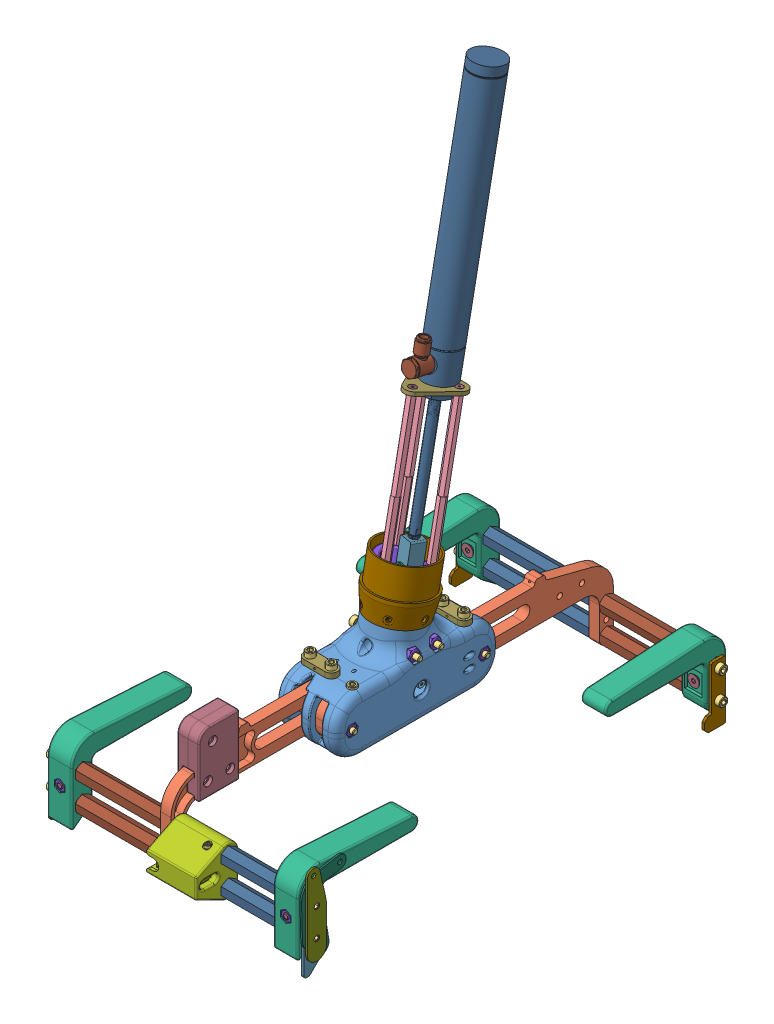
SolidWorks assembly 971-18-A-4000_The Claw, configuration Default. Lengths in mm. (continued)
Mates (geometry in assembly coordinates): (continued)
- Concentric85: concentric anti-aligned: cylinder of 971-18-P-0153_Claw Piston Mount-1 through (0 214.9449 -23.313) axis (0 0.981514 -0.19139) radius 1.632; cylinder of FHCS-19 through (0 208.7122 -22.0976) axis (0 -0.981514 0.19139) radius 1.4224
- Coincident109: coincident aligned: plane of 971-18-P-0153_Claw Piston Mount-1 through (-15.7499 209.7238 -50.0883) normal (0 0.981514 -0.19139); plane of FHCS-19 through (-1.3527 214.8607 -23.7448) normal (0 0.981514 -0.19139)
- Concentric90: concentric anti-aligned: cylinder of Bearings-1 through (15.2468 27.94 -18.3873) axis (1 0 0) radius 4.7625; cylinder of 971-18-P-0120_Printed Claw Pulley-4 through (0.264 27.94 -18.3873) axis (-1 0 0) radius 4.7625
- Coincident116: coincident anti-aligned: plane of Bearings-1 through (7.7788 27.5507 -23.1339) normal (-1 0 0); plane of 971-18-P-0120_Printed Claw Pulley-4 through (7.7788 31.7428 -18.1529) normal (1 0 0)
- Coincident117: coincident anti-aligned: plane of Bearings-2 through (-11.0808 23.5364 -0.7924) normal (-1 0 0); plane of 971-18-P-0120_Printed Claw Pulley-3 through (-11.0808 29.7802 -2.3147) normal (1 0 0)
- Concentric91: concentric anti-aligned: cylinder of Bearings-2 through (-3.6127 27.94 1.0215) axis (1 0 0) radius 4.7625; cylinder of 971-18-P-0120_Printed Claw Pulley-3 through (-18.5955 27.94 1.0215) axis (-1 0 0) radius 4.7625
- Concentric1168: concentric aligned: cone of 971-18-P-0108_Printed Claw Body-1 through (-11.1125 53.5447 9.169) axis (0.5 -0.165748 -0.850016); cone of 93365A142_BRASS HEAT-SET INSERT FOR PLASTICS-1 through (-10.8148 53.446 8.663) axis (0.5 -0.165748 -0.850016)
- Tangent1: tangent aligned: cylinder of 971-18-P-0108_Printed Claw Body-1 through (0 43.6283 -8.5073) axis (0 0.981514 -0.19139) radius 22.225; plane of 93365A142_BRASS HEAT-SET INSERT FOR PLASTICS-1 through (-11.1125 53.5447 9.169) normal (-0.5 0.165748 0.850016)
- Concentric1169: concentric aligned: cone of 971-18-P-0108_Printed Claw Body-1 through (-22.225 49.8609 -9.7226) axis (1 0 0); cone of 93365A142_BRASS HEAT-SET INSERT FOR PLASTICS-2 through (-21.6297 49.8609 -9.7226) axis (1 0 0)
- Tangent2: tangent aligned: cylinder of 971-18-P-0108_Printed Claw Body-1 through (0 43.6283 -8.5073) axis (0 0.981514 -0.19139) radius 22.225; plane of 93365A142_BRASS HEAT-SET INSERT FOR PLASTICS-2 through (-22.225 49.8609 -9.7226) normal (-1 0 0)
- Concentric1170: concentric aligned: cone of 971-18-P-0108_Printed Claw Body-1 through (-11.1125 46.1772 -28.6142) axis (0.5 0.165748 0.850016); cone of 93365A142_BRASS HEAT-SET INSERT FOR PLASTICS-4 through (-10.8148 46.2758 -28.1082) axis (0.5 0.165748 0.850016)
- Tangent3: tangent aligned: cylinder of 971-18-P-0108_Printed Claw Body-1 through (0 43.6283 -8.5073) axis (0 0.981514 -0.19139) radius 22.225; plane of 93365A142_BRASS HEAT-SET INSERT FOR PLASTICS-4 through (-11.1125 46.1772 -28.6142) normal (-0.5 -0.165748 -0.850016)
- Concentric1171: concentric aligned: cone of 971-18-P-0108_Printed Claw Body-1 through (11.1125 46.1772 -28.6142) axis (-0.5 0.165748 0.850016); cone of 93365A142_BRASS HEAT-SET INSERT FOR PLASTICS-6 through (10.8148 46.2758 -28.1082) axis (-0.5 0.165748 0.850016)
- Tangent4: tangent aligned: cylinder of 971-18-P-0108_Printed Claw Body-1 through (0 43.6283 -8.5073) axis (0 0.981514 -0.19139) radius 22.225; plane of 93365A142_BRASS HEAT-SET INSERT FOR PLASTICS-6 through (11.1125 46.1772 -28.6142) normal (0.5 -0.165748 -0.850016)
- Concentric1172: concentric aligned: cone of 971-18-P-0108_Printed Claw Body-1 through (22.225 49.8609 -9.7226) axis (-1 0 0); cone of 93365A142_BRASS HEAT-SET INSERT FOR PLASTICS-8 through (21.6297 49.8609 -9.7226) axis (-1 0 0)
- Tangent5: tangent aligned: cylinder of 971-18-P-0108_Printed Claw Body-1 through (0 43.6283 -8.5073) axis (0 0.981514 -0.19139) radius 22.225; plane of 93365A142_BRASS HEAT-SET INSERT FOR PLASTICS-8 through (22.225 49.8609 -9.7226) normal (1 0 0)
- Concentric1173: concentric aligned: cone of 971-18-P-0108_Printed Claw Body-1 through (11.1125 53.5447 9.169) axis (-0.5 -0.165748 -0.850016); cone of 93365A142_BRASS HEAT-SET INSERT FOR PLASTICS-10 through (10.8148 53.446 8.663) axis (-0.5 -0.165748 -0.850016)
- Tangent6: tangent aligned: cylinder of 971-18-P-0108_Printed Claw Body-1 through (0 43.6283 -8.5073) axis (0 0.981514 -0.19139) radius 22.225; plane of 93365A142_BRASS HEAT-SET INSERT FOR PLASTICS-10 through (11.1125 53.5447 9.169) normal (0.5 0.165748 0.850016)
- Tangent7: tangent: cylinder of 971-18-P-0108_Printed Claw Body-1 through (-25.2095 0 36.5125) axis (1 0 0) radius 3.175; torus of 9433K640_PRECISION STAINLESS STEEL EXTENSION SPRING-2
- Concentric1202: concentric anti-aligned: circle of 92311A433_18-8 SS CUP POINT SET SCREW-11; circle of 971-18-P-0077_Main Claw plate-2
- Concentric1206: concentric anti-aligned: circle of 92311A433_18-8 SS CUP POINT SET SCREW-14; circle of 971-18-P-0077_Main Claw plate-2
- Concentric1207: concentric anti-aligned: circle of SHCS-43; circle of 92311A433_18-8 SS CUP POINT SET SCREW-11
- Concentric1215: concentric anti-aligned: cylinder of SHCS-12 through (-19.177 30.1625 50.8) axis (0 -1 0) radius 2.413; circle of 94638A222_NYLON UNTHREADED SPACERS-1
- Width22: width anti-aligned: plane of 94638A222_NYLON UNTHREADED SPACERS-1 through (-19.177 16.6687 50.8) normal (0 1 0); plane of 971-18-P-0108_Printed Claw Body-1 through (-19.177 -16.6687 50.8) normal (0 -1 0); plane of 94638A222_NYLON UNTHREADED SPACERS-1 through (3.81 17.4625 -74.6125) normal (0 -1 0); plane of 971-18-P-0108_Printed Claw Body-1 through (3.81 -17.4625 -74.6125) normal (0 1 0)
- Concentric1216: concentric anti-aligned: cylinder of SHCS-3 through (-19.177 22.225 -50.8) axis (0 -1 0) radius 2.413; circle of 94638A222_NYLON UNTHREADED SPACERS-2
- Width23: width anti-aligned: plane of 94638A222_NYLON UNTHREADED SPACERS-2 through (-19.177 16.6687 -50.8) normal (0 1 0); plane of 971-18-P-0108_Printed Claw Body-1 through (-19.177 -16.6687 -50.8) normal (0 -1 0); plane of 94638A222_NYLON UNTHREADED SPACERS-2 through (3.81 17.4625 -74.6125) normal (0 -1 0); plane of 971-18-P-0108_Printed Claw Body-1 through (3.81 -17.4625 -74.6125) normal (0 1 0)
- Concentric1217: concentric anti-aligned: cylinder of SHCS-11 through (0 30.1625 50.8) axis (0 -1 0) radius 2.413; circle of 94639A586_NYLON UNTHREADED SPACERS-3
- Width25: width anti-aligned: plane of 94639A586_NYLON UNTHREADED SPACERS-3 through (0 -6.7469 50.8) normal (0 1 0); plane of 971-18-P-0108_Printed Claw Body-1 through (0 -17.0656 50.8) normal (0 -1 0); plane of 94639A586_NYLON UNTHREADED SPACERS-3 through (0 -6.35 50.8) normal (0 -1 0); plane of 971-18-P-0108_Printed Claw Body-1 through (3.81 -17.4625 -74.6125) normal (0 1 0)
- Concentric1218: concentric anti-aligned: cylinder of SHCS-11 through (0 30.1625 50.8) axis (0 -1 0) radius 2.413; circle of 94639A586_NYLON UNTHREADED SPACERS-1
- Width26: width anti-aligned: plane of 94639A586_NYLON UNTHREADED SPACERS-1 through (0 17.0656 50.8) normal (0 1 0); plane of 971-18-P-0108_Printed Claw Body-1 through (0 6.7469 50.8) normal (0 -1 0); plane of 94639A586_NYLON UNTHREADED SPACERS-1 through (3.81 17.4625 -74.6125) normal (0 -1 0); plane of 971-18-P-0108_Printed Claw Body-1 through (0 6.35 50.8) normal (0 1 0)
- Concentric1219: concentric anti-aligned: cylinder of SHCS-8 through (0 30.1625 -50.8) axis (0 -1 0) radius 2.413; circle of 94639A586_NYLON UNTHREADED SPACERS-4
- Width27: width aligned: plane of 94639A586_NYLON UNTHREADED SPACERS-4 through (0 -6.7469 -50.8) normal (0 1 0); plane of 971-18-P-0108_Printed Claw Body-1 through (0 -17.0656 -50.8) normal (0 -1 0); plane of 94639A586_NYLON UNTHREADED SPACERS-4 through (3.81 -17.4625 -74.6125) normal (0 1 0); plane of 971-18-P-0108_Printed Claw Body-1 through (0 -6.35 -50.8) normal (0 -1 0)
- Concentric1220: concentric anti-aligned: cylinder of SHCS-8 through (0 30.1625 -50.8) axis (0 -1 0) radius 2.413; circle of 94639A586_NYLON UNTHREADED SPACERS-2
- Width28: width anti-aligned: plane of 94639A586_NYLON UNTHREADED SPACERS-2 through (0 17.0656 -50.8) normal (0 1 0); plane of 971-18-P-0108_Printed Claw Body-1 through (0 6.7469 -50.8) normal (0 -1 0); plane of 94639A586_NYLON UNTHREADED SPACERS-2 through (3.81 17.4625 -74.6125) normal (0 -1 0); plane of 971-18-P-0108_Printed Claw Body-1 through (0 6.35 -50.8) normal (0 1 0)
- Concentric1221: concentric anti-aligned: cylinder of SHCS-10 through (19.177 22.225 50.8) axis (0 -1 0) radius 2.413; circle of 94638A222_NYLON UNTHREADED SPACERS-4
- Concentric1222: concentric anti-aligned: cylinder of SHCS-9 through (19.177 30.1625 -50.8) axis (0 -1 0) radius 2.413; circle of 94638A222_NYLON UNTHREADED SPACERS-3
- Width29: width anti-aligned: plane of 94638A222_NYLON UNTHREADED SPACERS-3 through (19.177 16.6687 -50.8) normal (0 1 0); plane of 971-18-P-0108_Printed Claw Body-1 through (19.177 -16.6687 -50.8) normal (0 -1 0); plane of 94638A222_NYLON UNTHREADED SPACERS-3 through (3.81 17.4625 -74.6125) normal (0 -1 0); plane of 971-18-P-0108_Printed Claw Body-1 through (3.81 -17.4625 -74.6125) normal (0 1 0)
- Width30: width anti-aligned: plane of 94638A222_NYLON UNTHREADED SPACERS-4 through (19.177 -16.6687 50.8) normal (0 -1 0); plane of 971-18-P-0108_Printed Claw Body-1 through (19.177 16.6687 50.8) normal (0 1 0); plane of 94638A222_NYLON UNTHREADED SPACERS-4 through (3.81 -17.4625 -74.6125) normal (0 1 0); plane of 971-18-P-0108_Printed Claw Body-1 through (3.81 17.4625 -74.6125) normal (0 -1 0)
- Concentric1223: concentric anti-aligned: cylinder of SHCS-2 through (-25.4 0 60.325) axis (1 0 0) radius 2.413; circle of 94639A550_NYLON UNTHREADED SPACERS-3
- Width31: width anti-aligned: plane of 94639A550_NYLON UNTHREADED SPACERS-3 through (-4.6673 0 60.325) normal (1 0 0); plane of 971-18-P-0108_Printed Claw Body-1 through (-14.1922 0 60.325) normal (-1 0 0); plane of 94639A550_NYLON UNTHREADED SPACERS-3 through (-3.81 17.4625 -74.6125) normal (-1 0 0); plane of 971-18-P-0108_Printed Claw Body-1 through (-15.0495 17.4625 -74.6125) normal (1 0 0)
- Concentric1224: concentric anti-aligned: cylinder of SHCS-2 through (-25.4 0 60.325) axis (1 0 0) radius 2.413; circle of 94639A550_NYLON UNTHREADED SPACERS-4
- Width32: width anti-aligned: plane of 94639A550_NYLON UNTHREADED SPACERS-4 through (4.6673 0 60.325) normal (-1 0 0); plane of 971-18-P-0108_Printed Claw Body-1 through (14.1922 0 60.325) normal (1 0 0); plane of 94639A550_NYLON UNTHREADED SPACERS-4 through (3.81 17.4625 -74.6125) normal (1 0 0); plane of 971-18-P-0108_Printed Claw Body-1 through (15.0495 17.4625 -74.6125) normal (-1 0 0)
- Concentric1225: concentric aligned: cylinder of SHCS-1 through (-25.4 0 -60.325) axis (1 0 0) radius 2.413; circle of 94639A550_NYLON UNTHREADED SPACERS-1
- Width33: width anti-aligned: plane of 94639A550_NYLON UNTHREADED SPACERS-1 through (-14.1922 0 -60.325) normal (-1 0 0); plane of 971-18-P-0108_Printed Claw Body-1 through (-4.6673 0 -60.325) normal (1 0 0); plane of 94639A550_NYLON UNTHREADED SPACERS-1 through (-15.0495 17.4625 -74.6125) normal (1 0 0); plane of 971-18-P-0108_Printed Claw Body-1 through (-3.81 17.4625 -74.6125) normal (-1 0 0)
- Concentric1226: concentric anti-aligned: cylinder of SHCS-1 through (-25.4 0 -60.325) axis (1 0 0) radius 2.413; circle of 94639A550_NYLON UNTHREADED SPACERS-2
- Width34: width aligned: plane of 94639A550_NYLON UNTHREADED SPACERS-2 through (4.6673 0 -60.325) normal (-1 0 0); plane of 971-18-P-0108_Printed Claw Body-1 through (14.1922 0 -60.325) normal (1 0 0); plane of 94639A550_NYLON UNTHREADED SPACERS-2 through (15.0495 17.4625 -74.6125) normal (-1 0 0); plane of 971-18-P-0108_Printed Claw Body-1 through (3.81 17.4625 -74.6125) normal (1 0 0)
- Concentric1236: concentric aligned: circle of 971-18-P-0077_Main Claw plate-3; circle of 92311A433_18-8 SS CUP POINT SET SCREW-5
- Concentric1238: concentric anti-aligned: circle of 971-18-P-0077_Main Claw plate-3; circle of 92311A433_18-8 SS CUP POINT SET SCREW-1
- Concentric1275: concentric aligned: circle of 91780A049_ALUM FEM THRDED HEX STANDOFF-2; circle of 98637A123_ALLOY STEEL MIL SPEC CUP POINT SET SCREW-3
- Concentric1276: concentric aligned: circle of 91780A049_ALUM FEM THRDED HEX STANDOFF-5; circle of 98637A123_ALLOY STEEL MIL SPEC CUP POINT SET SCREW-3
- Coincident286: coincident anti-aligned: plane of 91780A049_ALUM FEM THRDED HEX STANDOFF-2 through (17.26 132.4555 -31.6177) normal (0 0.981514 -0.19139); plane of 91780A049_ALUM FEM THRDED HEX STANDOFF-5 through (18.7431 132.2213 -32.8189) normal (0 -0.981514 0.19139)
- Concentric1277: concentric anti-aligned: circle of 91780A049_ALUM FEM THRDED HEX STANDOFF-3; circle of 98637A123_ALLOY STEEL MIL SPEC CUP POINT SET SCREW-2
- Concentric1278: concentric aligned: circle of 91780A049_ALUM FEM THRDED HEX STANDOFF-4; circle of 98637A123_ALLOY STEEL MIL SPEC CUP POINT SET SCREW-2
- Coincident287: coincident anti-aligned: plane of 91780A049_ALUM FEM THRDED HEX STANDOFF-3 through (-15.7499 131.1145 -38.4951) normal (0 -0.981514 0.19139); plane of 91780A049_ALUM FEM THRDED HEX STANDOFF-4 through (-12.0838 131.8123 -34.9162) normal (0 0.981514 -0.19139)
- Concentric1279: concentric anti-aligned: circle of 98637A123_ALLOY STEEL MIL SPEC CUP POINT SET SCREW-1; circle of 91780A049_ALUM FEM THRDED HEX STANDOFF-6
- Concentric1280: concentric anti-aligned: circle of 91780A049_ALUM FEM THRDED HEX STANDOFF-1; circle of 98637A123_ALLOY STEEL MIL SPEC CUP POINT SET SCREW-1
- Coincident289: coincident anti-aligned: plane of 91780A049_ALUM FEM THRDED HEX STANDOFF-1 through (-3.5893 137.1801 -7.3885) normal (0 -0.981514 0.19139); plane of 91780A049_ALUM FEM THRDED HEX STANDOFF-6 through (1.8331 137.6448 -5.0051) normal (0 0.981514 -0.19139)
- Concentric1281: concentric anti-aligned: cylinder of FHCS-17 through (0 208.7122 -22.0976) axis (0 -0.981514 0.19139) radius 1.4224; circle of 91780A049_ALUM FEM THRDED HEX STANDOFF-6
- Coincident291: coincident anti-aligned: plane of 971-18-P-0153_Claw Piston Mount-1 through (-15.7499 206.6075 -49.4806) normal (0 -0.981514 0.19139); plane of 91780A049_ALUM FEM THRDED HEX STANDOFF-1 through (-3.5893 211.9715 -21.9724) normal (0 0.981514 -0.19139)
- Concentric1282: concentric anti-aligned: circle of FHCS-18; circle of 91780A049_ALUM FEM THRDED HEX STANDOFF-5
- Coincident293: coincident anti-aligned: plane of 971-18-P-0153_Claw Piston Mount-1 through (-15.7499 206.6075 -49.4806) normal (0 -0.981514 0.19139); plane of 91780A049_ALUM FEM THRDED HEX STANDOFF-5 through (18.7431 207.0127 -47.4028) normal (0 0.981514 -0.19139)
- Concentric1283: concentric anti-aligned: circle of FHCS-15; circle of 91780A049_ALUM FEM THRDED HEX STANDOFF-3
- Coincident294: coincident anti-aligned: plane of 971-18-P-0153_Claw Piston Mount-1 through (-15.7499 206.6075 -49.4806) normal (0 -0.981514 0.19139); plane of 91780A049_ALUM FEM THRDED HEX STANDOFF-3 through (-15.7499 205.9058 -53.079) normal (0 0.981514 -0.19139)
- Concentric1310: concentric anti-aligned: cylinder of Beam Diffuse Sensor-1 through (30.5617 -48.646 194.183) axis (0 1 0) radius 1.524; cylinder of SHCS-26 through (30.5617 -24.389 194.183) axis (0 -1 0) radius 1.4224
- Concentric1313: concentric aligned: cylinder of 94639A550_NYLON UNTHREADED SPACERS-4 through (4.6673 0 60.325) axis (1 0 0) radius 6.35; cylinder of 94639A550_NYLON UNTHREADED SPACERS-3 through (-14.1922 0 60.325) axis (1 0 0) radius 6.35
- Concentric1314: concentric aligned: cylinder of SHCS-37 through (116.3637 -29.5056 -185.7375) axis (-1 0 0) radius 2.413; cylinder of 971-18-P-0299_Printed Claw Ends-1 through (114.0778 -29.5056 -185.7375) axis (-1 0 0) radius 2.4892
- Concentric1315: concentric aligned: cylinder of SHCS-39 through (116.3637 -54.9056 -185.7375) axis (-1 0 0) radius 2.413; cylinder of 971-18-P-0299_Printed Claw Ends-1 through (114.0778 -54.9056 -185.7375) axis (-1 0 0) radius 2.4892
- Concentric1316: concentric anti-aligned: cylinder of SHCS-43 through (-116.3637 -29.5056 -185.7375) axis (1 0 0) radius 2.413; cylinder of 971-18-P-0299_Printed Claw Ends-2 through (-91.8528 -29.5056 -185.7375) axis (-1 0 0) radius 2.4892
- Concentric1317: concentric anti-aligned: cylinder of SHCS-41 through (-116.3637 -54.9056 -185.7375) axis (1 0 0) radius 2.413; cylinder of 971-18-P-0299_Printed Claw Ends-2 through (-91.8528 -54.9056 -185.7375) axis (-1 0 0) radius 2.4892
- Concentric1318: concentric aligned: cylinder of SHCS-24 through (-116.3637 -29.5056 185.7375) axis (1 0 0) radius 2.413; cylinder of 971-18-P-0299_Printed Claw Ends-3 through (-114.0778 -29.5056 185.7375) axis (1 0 0) radius 2.4892
- Concentric1319: concentric aligned: cylinder of SHCS-44 through (-116.3637 -54.9056 185.7375) axis (1 0 0) radius 2.413; cylinder of 971-18-P-0299_Printed Claw Ends-3 through (-114.0778 -54.9056 185.7375) axis (1 0 0) radius 2.4892
- Concentric1321: concentric anti-aligned: cylinder of SHCS-33 through (116.3637 -29.5056 185.7375) axis (-1 0 0) radius 2.413; cylinder of 971-18-P-0299_Printed Claw Ends-4 through (91.8528 -29.5056 185.7375) axis (1 0 0) radius 2.4892
- Concentric1322: concentric anti-aligned: cylinder of SHCS-35 through (116.3637 -54.9056 185.7375) axis (-1 0 0) radius 2.413; cylinder of 971-18-P-0299_Printed Claw Ends-4 through (91.8528 -54.9056 185.7375) axis (1 0 0) radius 2.4892
- Coincident363: coincident anti-aligned: plane of 971-18-P-0077_Main Claw plate-3 through (-4.6673 -158.75 26.9875) normal (1 0 0); plane of 971-18-P-0300_Printed Claw Beam Break Mount-1 through (-4.6673 -29.469 185.801) normal (-1 0 0)
- Coincident365: coincident anti-aligned: plane of Beam Diffuse Sensor-1 through (2.3678 -48.646 191.135) normal (0 0 -1); plane of 971-18-P-0300_Printed Claw Beam Break Mount-1 through (-4.6673 -35.692 191.135) normal (0 0 1)
- Coincident366: coincident anti-aligned: plane of Beam Diffuse Sensor-1 through (2.3678 -48.646 191.135) normal (0 -1 0); plane of 971-18-P-0300_Printed Claw Beam Break Mount-1 through (-4.6673 -48.646 191.135) normal (0 1 0)
- Coincident367: coincident anti-aligned: plane of Beam Diffuse Sensor-1 through (34.0678 -48.646 212.217) normal (1 0 0); plane of 971-18-P-0300_Printed Claw Beam Break Mount-1 through (34.0678 -35.819 225.3308) normal (-1 0 0)
- Coincident368: coincident anti-aligned: plane of SHCS-26 through (31.0198 -24.389 192.0498) normal (0 -1 0); plane of 971-18-P-0300_Printed Claw Beam Break Mount-1 through (30.5626 -24.389 194.183) normal (0 1 0)
- Concentric1324: concentric anti-aligned: cylinder of 971-18-P-0299_Printed Claw Ends-4 through (102.9652 -42.2056 195.2625) axis (0 0 -1) radius 2.4892; cylinder of FHCS-20 through (102.9652 -42.2056 195.2625) axis (0 0 1) radius 2.413
- Concentric1325: concentric anti-aligned: cylinder of Nylon-Insert Locknut-22 through (102.9652 -42.2056 188.087) axis (0 0 -1) radius 2.413; cylinder of FHCS-20 through (102.9652 -42.2056 195.2625) axis (0 0 1) radius 2.413
- Coincident373: coincident anti-aligned: plane of 971-18-P-0299_Printed Claw Ends-4 through (102.9652 -29.5056 190.5) normal (0 0 1); plane of Nylon-Insert Locknut-22 through (103.2706 -47.6964 190.5) normal (0 0 -1)
- Coincident374: coincident aligned: plane of 971-18-P-0299_Printed Claw Ends-4 through (91.8528 -26.9529 176.2125) normal (0 0 -1); plane of FHCS-20 through (103.8895 -44.4346 176.2125) normal (0 0 -1)
- Concentric1327: concentric anti-aligned: cylinder of 971-18-P-0299_Printed Claw Ends-3 through (-102.9652 -42.2056 195.2625) axis (0 0 -1) radius 2.4892; cylinder of FHCS-21 through (-102.9652 -42.2056 195.2625) axis (0 0 1) radius 2.413
- Coincident375: coincident aligned: plane of 971-18-P-0299_Printed Claw Ends-3 through (-114.0778 -26.9529 176.2125) normal (0 0 -1); plane of FHCS-21 through (-101.7917 -44.314 176.2125) normal (0 0 -1)
- Coincident376: coincident aligned: plane of 971-18-P-0299_Printed Claw Ends-2 through (-91.8528 -26.9529 -176.2125) normal (0 0 1); plane of FHCS-24 through (-105.3759 -42.0994 -176.2125) normal (0 0 1)
- Concentric1328: concentric anti-aligned: cylinder of 971-18-P-0299_Printed Claw Ends-2 through (-102.9652 -42.2056 -195.2625) axis (0 0 1) radius 2.4892; cylinder of FHCS-24 through (-102.9652 -42.2056 -195.2625) axis (0 0 -1) radius 2.413
- Concentric1329: concentric anti-aligned: cylinder of 971-18-P-0299_Printed Claw Ends-1 through (102.9652 -42.2056 -195.2625) axis (0 0 1) radius 2.4892; cylinder of FHCS-26 through (102.9652 -42.2056 -195.2625) axis (0 0 -1) radius 2.413
- Coincident377: coincident aligned: plane of 971-18-P-0299_Printed Claw Ends-1 through (114.0778 -26.9529 -176.2125) normal (0 0 1); plane of FHCS-26 through (100.5728 -42.5196 -176.2125) normal (0 0 1)
- Concentric1330: concentric anti-aligned: cylinder of FHCS-21 through (-102.9652 -42.2056 195.2625) axis (0 0 1) radius 2.413; cylinder of Nylon-Insert Locknut-23 through (-102.9652 -42.2056 188.087) axis (0 0 -1) radius 2.413
- Coincident378: coincident anti-aligned: plane of 971-18-P-0299_Printed Claw Ends-3 through (-102.9652 -29.5056 190.5) normal (0 0 1); plane of Nylon-Insert Locknut-23 through (-102.033 -47.6253 190.5) normal (0 0 -1)
- Concentric1331: concentric anti-aligned: cylinder of FHCS-24 through (-102.9652 -42.2056 -195.2625) axis (0 0 -1) radius 2.413; cylinder of Nylon-Insert Locknut-25 through (-102.9652 -42.2056 -188.087) axis (0 0 1) radius 2.413
- Coincident379: coincident anti-aligned: plane of 971-18-P-0299_Printed Claw Ends-2 through (-102.9652 -29.5056 -190.5) normal (0 0 -1); plane of Nylon-Insert Locknut-25 through (-108.2293 -43.7966 -190.5) normal (0 0 1)
- Concentric1332: concentric anti-aligned: cylinder of FHCS-26 through (102.9652 -42.2056 -195.2625) axis (0 0 -1) radius 2.413; cylinder of Nylon-Insert Locknut-27 through (102.9652 -42.2056 -188.087) axis (0 0 1) radius 2.413
- Coincident380: coincident anti-aligned: plane of 971-18-P-0299_Printed Claw Ends-1 through (102.9652 -29.5056 -190.5) normal (0 0 -1); plane of Nylon-Insert Locknut-27 through (98.0574 -44.6866 -190.5) normal (0 0 1)
- Concentric1336: concentric anti-aligned: cylinder of 971-18-P-0108_Printed Claw Body-1 through (0 -22.2934 4.3471) axis (0 0.981514 -0.19139) radius 14.2875; cylinder of 971-18-P-0304_Claw Standoff Ring-1 through (0 84.2529 -16.4288) axis (0 -0.981514 0.19139) radius 15.875
- Coincident388: coincident anti-aligned: plane of 91780A049_ALUM FEM THRDED HEX STANDOFF-6 through (1.8331 62.8535 9.5788) normal (0 0.19139 0.981514); plane of 971-18-P-0304_Claw Standoff Ring-1 through (-1.8331 88.3546 4.6062) normal (0 -0.19139 -0.981514)
- Coincident389: coincident anti-aligned: plane of 91780A049_ALUM FEM THRDED HEX STANDOFF-6 through (-1.8331 62.8535 9.5788) normal (-0.866025 0.095695 0.490757); plane of 971-18-P-0304_Claw Standoff Ring-1 through (-3.6662 87.7469 1.4899) normal (0.866025 -0.095695 -0.490757)
- Concentric1337: concentric anti-aligned: cylinder of 971-18-P-0299_Printed Claw Ends-4 through (91.8528 -29.5056 185.7375) axis (1 0 0) radius 2.4892; cylinder of 971-18-P-0312_Claw Fangs-1 through (116.3637 -29.5056 185.7375) axis (-1 0 0) radius 2.4892
- Concentric1338: concentric anti-aligned: cylinder of 971-18-P-0299_Printed Claw Ends-4 through (91.8528 -54.9056 185.7375) axis (1 0 0) radius 2.4892; cylinder of 971-18-P-0312_Claw Fangs-1 through (116.3637 -54.9056 185.7375) axis (-1 0 0) radius 2.4892
- Coincident390: coincident anti-aligned: plane of 971-18-P-0299_Printed Claw Ends-4 through (114.0778 -54.9056 185.7375) normal (1 0 0); plane of 971-18-P-0312_Claw Fangs-1 through (114.0778 -76.4956 200.7755) normal (-1 0 0)
- Coincident391: coincident anti-aligned: plane of SHCS-33 through (116.3637 -27.5183 188.8835) normal (-1 0 0); plane of 971-18-P-0312_Claw Fangs-1 through (116.3637 -76.4956 200.7755) normal (1 0 0)
- Coincident392: coincident anti-aligned: plane of SHCS-35 through (116.3637 -52.021 183.3869) normal (-1 0 0); plane of 971-18-P-0312_Claw Fangs-1 through (116.3637 -76.4956 200.7755) normal (1 0 0)
- Concentric1342: concentric aligned: cylinder of 971-18-P-0077_Main Claw plate-2 through (14.1922 -54.9056 -185.7375) axis (-1 0 0) radius 2.4892; cylinder of 971-18-P-0299_Printed Claw Ends-1 through (114.0778 -54.9056 -185.7375) axis (-1 0 0) radius 2.4892
- Concentric1344: concentric aligned: cylinder of 971-18-P-0077_Main Claw plate-3 through (-14.1922 -29.5056 185.7375) axis (1 0 0) radius 2.4892; cylinder of SHCS-24 through (-116.3637 -29.5056 185.7375) axis (1 0 0) radius 2.413
- Concentric1347: concentric anti-aligned: cylinder of 971-18-P-0299_Printed Claw Ends-2 through (-91.8528 -29.5056 -185.7375) axis (-1 0 0) radius 2.4892; cylinder of 971-18-P-0312_Claw Fangs-6 through (-116.3637 -29.5056 -185.7375) axis (1 0 0) radius 2.4892
- Concentric1348: concentric anti-aligned: cylinder of 971-18-P-0299_Printed Claw Ends-2 through (-91.8528 -54.9056 -185.7375) axis (-1 0 0) radius 2.4892; cylinder of 971-18-P-0312_Claw Fangs-6 through (-116.3637 -54.9056 -185.7375) axis (1 0 0) radius 2.4892
- Coincident396: coincident anti-aligned: plane of 971-18-P-0299_Printed Claw Ends-2 through (-114.0778 -54.9056 -185.7375) normal (-1 0 0); plane of 971-18-P-0312_Claw Fangs-6 through (-114.0778 -76.4956 -200.7755) normal (1 0 0)
- Coincident397: coincident anti-aligned: plane of SHCS-41 through (-116.3637 -58.3774 -187.0767) normal (1 0 0); plane of 971-18-P-0312_Claw Fangs-6 through (-116.3637 -76.4956 -200.7755) normal (-1 0 0)
- Coincident398: coincident anti-aligned: plane of SHCS-43 through (-116.3637 -28.7687 -189.3849) normal (1 0 0); plane of 971-18-P-0312_Claw Fangs-6 through (-116.3637 -76.4956 -200.7755) normal (-1 0 0)
- Concentric1354: concentric anti-aligned: cylinder of SHCS-37 through (116.3637 -29.5056 -185.7375) axis (-1 0 0) radius 2.413; cylinder of 971-18-P-0312_Claw Fangs-11 through (114.0778 -29.5056 -185.7375) axis (1 0 0) radius 2.4892
- Concentric1355: concentric anti-aligned: cylinder of SHCS-39 through (116.3637 -54.9056 -185.7375) axis (-1 0 0) radius 2.413; cylinder of 971-18-P-0312_Claw Fangs-11 through (114.0778 -54.9056 -185.7375) axis (1 0 0) radius 2.4892
- Coincident406: coincident anti-aligned: plane of 971-18-P-0299_Printed Claw Ends-1 through (114.0778 -54.9056 -185.7375) normal (1 0 0); plane of 971-18-P-0312_Claw Fangs-11 through (114.0778 -76.4956 -200.7755) normal (-1 0 0)
- Coincident407: coincident anti-aligned: plane of SHCS-39 through (116.3637 -52.4219 -188.5084) normal (-1 0 0); plane of 971-18-P-0312_Claw Fangs-11 through (116.3637 -76.4956 -200.7755) normal (1 0 0)
- Coincident408: coincident anti-aligned: plane of SHCS-37 through (116.3637 -25.7909 -185.9554) normal (-1 0 0); plane of 971-18-P-0312_Claw Fangs-11 through (116.3637 -76.4956 -200.7755) normal (1 0 0)
- Concentric1356: concentric anti-aligned: cylinder of SHCS-24 through (-116.3637 -29.5056 185.7375) axis (1 0 0) radius 2.413; cylinder of 971-18-P-0312_Claw Fangs-12 through (-114.0778 -29.5056 185.7375) axis (-1 0 0) radius 2.4892
- Concentric1357: concentric anti-aligned: cylinder of SHCS-44 through (-116.3637 -54.9056 185.7375) axis (1 0 0) radius 2.413; cylinder of 971-18-P-0312_Claw Fangs-12 through (-114.0778 -54.9056 185.7375) axis (-1 0 0) radius 2.4892
- Coincident409: coincident anti-aligned: plane of 971-18-P-0299_Printed Claw Ends-3 through (-114.0778 -54.9056 185.7375) normal (-1 0 0); plane of 971-18-P-0312_Claw Fangs-12 through (-114.0778 -76.4956 200.7755) normal (1 0 0)
- Coincident410: coincident anti-aligned: plane of SHCS-44 through (-116.3637 -54.2776 182.0698) normal (1 0 0); plane of 971-18-P-0312_Claw Fangs-12 through (-116.3637 -76.4956 200.7755) normal (-1 0 0)
- Coincident411: coincident anti-aligned: plane of SHCS-24 through (-116.3637 -33.1222 184.8619) normal (1 0 0); plane of 971-18-P-0312_Claw Fangs-12 through (-116.3637 -76.4956 200.7755) normal (-1 0 0)
- Concentric1360: concentric aligned: cylinder of SHCS-24 through (-116.3637 -29.5056 185.7375) axis (1 0 0) radius 2.413; circle of 971-18-P-0317_Claw Short Horizontal Standoff-4
- Coincident418: coincident anti-aligned: plane of 971-18-P-0299_Printed Claw Ends-3 through (-96.9327 -22.1733 185.7375) normal (0 -0.866025 -0.5); plane of 971-18-P-0317_Claw Short Horizontal Standoff-4 through (-14.1922 -22.1733 185.7375) normal (0 0.866025 0.5)
- Concentric1362: concentric anti-aligned: circle of 92311A433_18-8 SS CUP POINT SET SCREW-1; circle of 971-18-P-0317_Claw Short Horizontal Standoff-1
- Concentric1363: concentric aligned: circle of 92311A433_18-8 SS CUP POINT SET SCREW-5; circle of 971-18-P-0317_Claw Short Horizontal Standoff-4
- Coincident421: coincident anti-aligned: plane of 971-18-P-0077_Main Claw plate-3 through (-14.1922 -158.75 26.9875) normal (-1 0 0); plane of 971-18-P-0317_Claw Short Horizontal Standoff-4 through (-14.1922 -25.8394 192.0875) normal (1 0 0)
- Concentric1364: concentric anti-aligned: cylinder of SHCS-35 through (116.3637 -54.9056 185.7375) axis (-1 0 0) radius 2.413; circle of 971-18-P-0316_Claw Long Horizontal Standoff-4
- Coincident422: coincident anti-aligned: plane of 971-18-P-0299_Printed Claw Ends-4 through (96.9327 -29.5056 185.7375) normal (-1 0 0); plane of 971-18-P-0316_Claw Long Horizontal Standoff-4 through (96.9327 -58.5718 179.3875) normal (1 0 0)
- Concentric1365: concentric anti-aligned: cylinder of SHCS-33 through (116.3637 -29.5056 185.7375) axis (-1 0 0) radius 2.413; circle of 971-18-P-0316_Claw Long Horizontal Standoff-2
- Coincident423: coincident anti-aligned: plane of 971-18-P-0299_Printed Claw Ends-4 through (96.9327 -29.5056 185.7375) normal (-1 0 0); plane of 971-18-P-0316_Claw Long Horizontal Standoff-2 through (96.9327 -22.1733 185.7375) normal (1 0 0)
- Concentric1366: concentric aligned: circle of 92311A433_18-8 SS CUP POINT SET SCREW-5; circle of 971-18-P-0316_Claw Long Horizontal Standoff-2
- Concentric1367: concentric anti-aligned: circle of 92311A433_18-8 SS CUP POINT SET SCREW-1; circle of 971-18-P-0316_Claw Long Horizontal Standoff-4
- Coincident424: coincident anti-aligned: plane of 971-18-P-0077_Main Claw plate-3 through (-4.6673 -158.75 26.9875) normal (1 0 0); plane of 971-18-P-0316_Claw Long Horizontal Standoff-4 through (-4.6673 -58.5718 179.3875) normal (-1 0 0)
- Coincident425: coincident anti-aligned: plane of 971-18-P-0300_Printed Claw Beam Break Mount-1 through (-4.6673 -25.7661 179.3875) normal (0 0 1); plane of 971-18-P-0316_Claw Long Horizontal Standoff-2 through (-4.6673 -25.8394 179.3875) normal (0 0 -1)
- Coincident426: coincident anti-aligned: plane of 971-18-P-0300_Printed Claw Beam Break Mount-1 through (-4.6673 -33.1718 179.3875) normal (0 0.866025 0.5); plane of 971-18-P-0316_Claw Long Horizontal Standoff-2 through (-4.6673 -33.1718 179.3875) normal (0 -0.866025 -0.5)
- Coincident427: coincident anti-aligned: plane of 971-18-P-0299_Printed Claw Ends-4 through (96.9327 -22.1733 185.7375) normal (0 -0.866025 -0.5); plane of 971-18-P-0316_Claw Long Horizontal Standoff-2 through (-4.6673 -25.8394 192.0875) normal (0 0.866025 0.5)
- Coincident428: coincident anti-aligned: plane of 971-18-P-0299_Printed Claw Ends-4 through (96.9327 -47.5733 185.7375) normal (0 -0.866025 -0.5); plane of 971-18-P-0316_Claw Long Horizontal Standoff-4 through (-4.6673 -51.2394 192.0875) normal (0 0.866025 0.5)
- Coincident433: coincident anti-aligned: plane of 971-18-P-0299_Printed Claw Ends-1 through (96.9327 -51.2394 -192.0875) normal (0 0 1); plane of 971-18-P-0317_Claw Short Horizontal Standoff-2 through (14.1922 -51.2394 -192.0875) normal (0 0 -1)
- Concentric1370: concentric anti-aligned: circle of 92311A433_18-8 SS CUP POINT SET SCREW-14; circle of 971-18-P-0317_Claw Short Horizontal Standoff-2
- Concentric1371: concentric anti-aligned: circle of 92311A433_18-8 SS CUP POINT SET SCREW-11; circle of 971-18-P-0317_Claw Short Horizontal Standoff-3
- Coincident434: coincident anti-aligned: plane of 971-18-P-0077_Main Claw plate-2 through (14.1922 -158.75 -26.9875) normal (1 0 0); plane of 971-18-P-0317_Claw Short Horizontal Standoff-2 through (14.1922 -51.2394 -179.3875) normal (-1 0 0)
- Concentric1372: concentric anti-aligned: cylinder of SHCS-43 through (-116.3637 -29.5056 -185.7375) axis (1 0 0) radius 2.413; circle of 971-18-P-0316_Claw Long Horizontal Standoff-3
- Coincident435: coincident anti-aligned: plane of 971-18-P-0299_Printed Claw Ends-2 through (-96.9327 -29.5056 -185.7375) normal (1 0 0); plane of 971-18-P-0316_Claw Long Horizontal Standoff-3 through (-96.9327 -25.8394 -179.3875) normal (-1 0 0)
- Coincident436: coincident anti-aligned: plane of 971-18-P-0299_Printed Claw Ends-2 through (-96.9327 -25.8394 -179.3875) normal (0 -0.866025 -0.5); plane of 971-18-P-0316_Claw Long Horizontal Standoff-3 through (4.6673 -22.1733 -185.7375) normal (0 0.866025 0.5)
- Concentric1373: concentric anti-aligned: cylinder of SHCS-41 through (-116.3637 -54.9056 -185.7375) axis (1 0 0) radius 2.413; circle of 971-18-P-0316_Claw Long Horizontal Standoff-1
- Coincident437: coincident anti-aligned: plane of 971-18-P-0299_Printed Claw Ends-2 through (-96.9327 -29.5056 -185.7375) normal (1 0 0); plane of 971-18-P-0316_Claw Long Horizontal Standoff-1 through (-96.9327 -51.2394 -179.3875) normal (-1 0 0)
- Coincident438: coincident anti-aligned: plane of 971-18-P-0299_Printed Claw Ends-2 through (-96.9327 -51.2394 -179.3875) normal (0 -0.866025 -0.5); plane of 971-18-P-0316_Claw Long Horizontal Standoff-1 through (4.6673 -47.5733 -185.7375) normal (0 0.866025 0.5)
- Concentric1374: concentric anti-aligned: circle of 92311A433_18-8 SS CUP POINT SET SCREW-11; circle of 971-18-P-0316_Claw Long Horizontal Standoff-3
- Concentric1375: concentric anti-aligned: circle of 92311A433_18-8 SS CUP POINT SET SCREW-14; circle of 971-18-P-0316_Claw Long Horizontal Standoff-1
- Coincident439: coincident anti-aligned: plane of 971-18-P-0077_Main Claw plate-2 through (4.6673 -158.75 -26.9875) normal (-1 0 0); plane of 971-18-P-0316_Claw Long Horizontal Standoff-1 through (4.6673 -51.2394 -179.3875) normal (1 0 0)
- Coincident440: coincident anti-aligned: plane of 971-18-P-0299_Printed Claw Ends-3 through (-96.9327 -29.5056 185.7375) normal (1 0 0); plane of 971-18-P-0317_Claw Short Horizontal Standoff-1 through (-96.9327 -54.9056 185.7375) normal (-1 0 0)
- Coincident441: coincident anti-aligned: plane of 971-18-P-0299_Printed Claw Ends-3 through (-96.9327 -29.5056 185.7375) normal (1 0 0); plane of 971-18-P-0317_Claw Short Horizontal Standoff-4 through (-96.9327 -29.5056 185.7375) normal (-1 0 0)
- Concentric1376: concentric anti-aligned: cylinder of SHCS-44 through (-116.3637 -54.9056 185.7375) axis (1 0 0) radius 2.413; cylinder of 971-18-P-0317_Claw Short Horizontal Standoff-1 through (-14.1922 -54.9056 185.7375) axis (-1 0 0) radius 2.413
- Coincident442: coincident anti-aligned: plane of 971-18-P-0299_Printed Claw Ends-1 through (96.9327 -29.5056 -185.7375) normal (-1 0 0); plane of 971-18-P-0317_Claw Short Horizontal Standoff-3 through (96.9327 -29.5056 -185.7375) normal (1 0 0)
- Coincident443: coincident anti-aligned: plane of 971-18-P-0299_Printed Claw Ends-1 through (96.9327 -29.5056 -185.7375) normal (-1 0 0); plane of 971-18-P-0317_Claw Short Horizontal Standoff-2 through (96.9327 -54.9056 -185.7375) normal (1 0 0)
- Coincident444: coincident aligned: cylinder of SHCS-37 through (116.3637 -29.5056 -185.7375) axis (-1 0 0) radius 2.413; circle of 971-18-P-0317_Claw Short Horizontal Standoff-3
- Coincident456: coincident anti-aligned: plane of 971-18-P-0077_Main Claw plate-3 through (-14.1922 -158.75 26.9875) normal (-1 0 0); plane of 971-18-P-0318_Claw Pulley Mount-5 through (-14.1922 5.212 171.7608) normal (1 0 0)
- Coincident458: coincident aligned: plane of 971-18-P-0318_Claw Pulley Mount-5 through (-9.4298 29.9142 171.7608) normal (0 0 1); plane of 971-18-P-0318_Claw Pulley Mount-6 through (0.4127 29.9142 171.7608) normal (0 0 1)
- Coincident460: coincident anti-aligned: plane of 971-18-P-0077_Main Claw plate-3 through (-4.6673 -158.75 26.9875) normal (1 0 0); plane of 971-18-P-0318_Claw Pulley Mount-6 through (-4.6673 5.212 171.7608) normal (-1 0 0)
- Slot1: slot: cylinder of 94639A550_NYLON UNTHREADED SPACERS-3 through (-14.1922 0 60.325) axis (1 0 0) radius 6.35; cylinder of 971-18-P-0077_Main Claw plate-3 through (-14.1922 0 60.325) axis (1 0 0) radius 6.4135; cylinder of 971-18-P-0077_Main Claw plate-3 through (-4.6673 0 109.5375) axis (-1 0 0) radius 6.4135
- Slot2: slot: plane of 971-18-P-0077_Main Claw plate-3 through (-4.6673 -6.4135 -55.5625) normal (0 1 0); cylinder of 94639A550_NYLON UNTHREADED SPACERS-1 through (-4.6673 0 -60.325) axis (-1 0 0) radius 6.35; cylinder of 971-18-P-0077_Main Claw plate-3 through (-4.6673 0 -11.1125) axis (-1 0 0) radius 6.4135
- Slot3: slot: cylinder of 94639A550_NYLON UNTHREADED SPACERS-2 through (4.6673 0 -60.325) axis (1 0 0) radius 6.35; cylinder of 971-18-P-0077_Main Claw plate-2 through (14.1922 0 -60.325) axis (-1 0 0) radius 6.4135; cylinder of 971-18-P-0077_Main Claw plate-2 through (4.6673 0 -109.5375) axis (1 0 0) radius 6.4135
- Slot4: slot: cylinder of 94639A550_NYLON UNTHREADED SPACERS-4 through (4.6673 0 60.325) axis (1 0 0) radius 6.35; cylinder of 971-18-P-0077_Main Claw plate-2 through (14.1922 0 60.325) axis (-1 0 0) radius 6.4135; cylinder of 971-18-P-0077_Main Claw plate-2 through (4.6673 0 11.1125) axis (1 0 0) radius 6.4135
- Concentric1390: concentric anti-aligned: cylinder of 971-18-P-0077_Main Claw plate-2 through (14.1922 0 60.325) axis (-1 0 0) radius 6.4135; cylinder of 94639A550_NYLON UNTHREADED SPACERS-4 through (4.6673 0 60.325) axis (1 0 0) radius 6.35
- Coincident464: coincident aligned: plane of 971-18-P-0318_Claw Pulley Mount-5 through (-14.1922 14.6742 134.8544) normal (0 -0.96867 -0.248352); plane of 971-18-P-0318_Claw Pulley Mount-6 through (-4.6673 14.6742 134.8544) normal (0 -0.96867 -0.248352)
- Concentric1391: concentric anti-aligned: cylinder of SHCS-9 through (19.177 30.1625 -50.8) axis (0 -1 0) radius 2.413; cylinder of 971-18-P-0326_Claw Cable Holder-3 through (19.177 25.4 -50.8) axis (0 1 0) radius 2.4892
- Concentric1392: concentric anti-aligned: cylinder of SHCS-8 through (0 30.1625 -50.8) axis (0 -1 0) radius 2.413; cylinder of 971-18-P-0326_Claw Cable Holder-3 through (0 25.4 -50.8) axis (0 1 0) radius 2.4892
- Coincident467: coincident anti-aligned: plane of 971-18-P-0108_Printed Claw Body-1 through (28.575 25.4 74.6125) normal (0 1 0); plane of 971-18-P-0326_Claw Cable Holder-3 through (0 25.4 -50.8) normal (0 -1 0)
- Coincident468: coincident anti-aligned: plane of SHCS-8 through (-0.2642 30.1625 -47.0883) normal (0 -1 0); plane of 971-18-P-0326_Claw Cable Holder-3 through (0 30.1625 -50.8) normal (0 1 0)
- Coincident469: coincident anti-aligned: plane of SHCS-9 through (17.0378 30.1625 -47.7553) normal (0 -1 0); plane of 971-18-P-0326_Claw Cable Holder-3 through (0 30.1625 -50.8) normal (0 1 0)
- Concentric1393: concentric anti-aligned: cylinder of SHCS-11 through (0 30.1625 50.8) axis (0 -1 0) radius 2.413; cylinder of 971-18-P-0326_Claw Cable Holder-2 through (0 25.4 50.8) axis (0 1 0) radius 2.4892
- Concentric1394: concentric anti-aligned: cylinder of SHCS-12 through (-19.177 30.1625 50.8) axis (0 -1 0) radius 2.413; cylinder of 971-18-P-0326_Claw Cable Holder-2 through (-19.177 25.4 50.8) axis (0 1 0) radius 2.4892
- Coincident470: coincident anti-aligned: plane of 971-18-P-0108_Printed Claw Body-1 through (28.575 25.4 74.6125) normal (0 1 0); plane of 971-18-P-0326_Claw Cable Holder-2 through (-19.177 25.4 50.8) normal (0 -1 0)
- Coincident471: coincident anti-aligned: plane of SHCS-11 through (0.1511 30.1625 54.518) normal (0 -1 0); plane of 971-18-P-0326_Claw Cable Holder-2 through (-19.177 30.1625 50.8) normal (0 1 0)
- Coincident472: coincident anti-aligned: plane of SHCS-12 through (-19.0089 30.1625 47.0827) normal (0 -1 0); plane of 971-18-P-0326_Claw Cable Holder-2 through (-19.177 30.1625 50.8) normal (0 1 0)
- Concentric1395: concentric aligned: cylinder of SHCS-33 through (116.3637 -29.5056 185.7375) axis (-1 0 0) radius 3.9624; cylinder of 971-18-P-0361_Claw Fangs V2-1 through (116.3637 -29.5056 185.7375) axis (-1 0 0) radius 2.4892
- Coincident474: coincident anti-aligned: plane of 971-18-P-0299_Printed Claw Ends-4 through (114.0778 -54.9056 185.7375) normal (1 0 0); plane of 971-18-P-0361_Claw Fangs V2-1 through (114.0778 -29.5056 185.7375) normal (-1 0 0)
- Parallel9: parallel aligned: plane of 971-18-P-0299_Printed Claw Ends-4 through (91.8528 -23.3893 195.2625) normal (0 0 1); plane of 971-18-P-0361_Claw Fangs V2-1 through (116.3637 -86.6556 192.0875) normal (0 0 1)
- Concentric1396: concentric aligned: cylinder of SHCS-33 through (116.3637 -29.5056 185.7375) axis (-1 0 0) radius 3.9624; cylinder of 971-18-P-0367_Retrofit Fang Sheath-1 through (117.8877 -29.5056 185.7375) axis (-1 0 0) radius 4.9403
- Coincident475: coincident anti-aligned: plane of 971-18-P-0361_Claw Fangs V2-1 through (116.3637 -29.5056 185.7375) normal (1 0 0); plane of 971-18-P-0367_Retrofit Fang Sheath-1 through (116.3637 -66.6323 178.3564) normal (-1 0 0)
- Concentric1397: concentric aligned: cylinder of SHCS-33 through (116.3637 -29.5056 185.7375) axis (-1 0 0) radius 3.9624; cylinder of 971-18-P-0368_Retrofit Fang Sheath Outside-1 through (121.8565 -29.5056 185.7375) axis (-1 0 0) radius 2.4892
- Concentric1398: concentric aligned: cylinder of SHCS-35 through (116.3637 -54.9056 185.7375) axis (-1 0 0) radius 3.9624; cylinder of 971-18-P-0368_Retrofit Fang Sheath Outside-1 through (121.8565 -54.9056 185.7375) axis (-1 0 0) radius 2.4892
- Distance7: distance = 3.9688 mm anti-aligned: plane of 971-18-P-0361_Claw Fangs V2-1 through (116.3637 -29.5056 185.7375) normal (1 0 0); plane of 971-18-P-0368_Retrofit Fang Sheath Outside-1 through (120.3325 -64.0126 185.7375) normal (-1 0 0)
